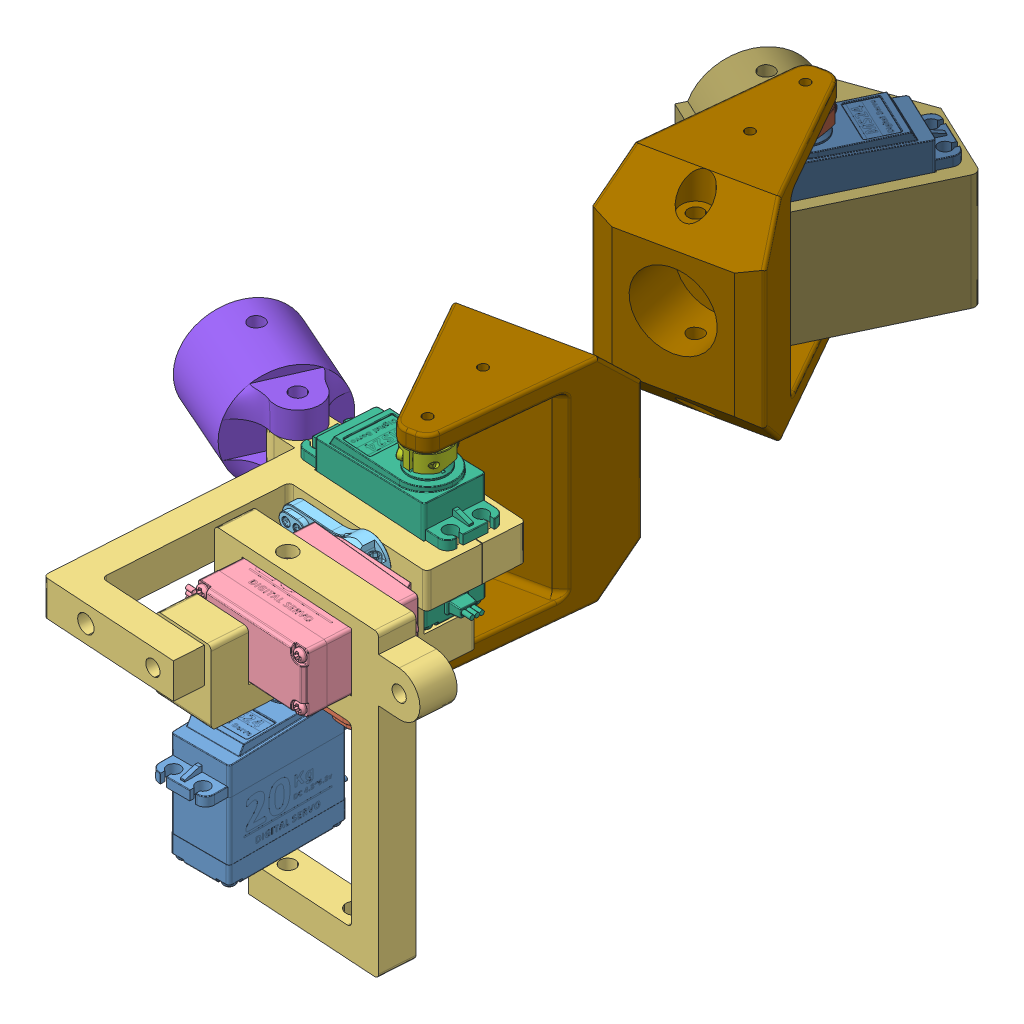
SolidWorks assembly Hip 2, configuration Default. Lengths in mm.
Overall size (141.38 121.48 305.42).
14 component instances, 12 part files, 42 mates.
Components (placement in the parent):
- Copy of DS3218MG MS24 Digital Servo 270^Hip 2-1: Copy of DS3218MG MS24 Digital Servo 270^Hip 2 [Default] at origin size (20.1 45.99 55.6) (virtual)
- Copy of Servo Arm^Hip 2-1: Copy of Servo Arm^Hip 2 [Default] x (-0.063067 0 0.998009) z (-0.998009 0 -0.063067) size (14.5 6.95 35.53) (virtual)
- Servo Connector-1: Servo Connector [Default] at (9.9951 39.015 0.6316) x (-0.998009 0 -0.063067) z (0 -1 0) size (75.07 39.5 102.5)
- Copy (3) of DS3218MG MS24 Digital Servo 270^Hip 2-1: Copy (3) of DS3218MG MS24 Digital Servo 270^Hip 2 [Default] at (0.3934 39.015 -5.9871) x (0 -1 0) z (0.998009 0 0.063067) size (20.1 45.99 55.6) (virtual)
- Copy (3) of Servo Arm^Hip 2-1: Copy (3) of Servo Arm^Hip 2 [Default] at (0.3934 39.015 -5.9871) x (0 -1 0) z (0.998009 0 0.063067) size (14.5 6.95 35.53) (virtual)
- Servo Connector-2: Servo Connector [Default] at (-7.1411 39.015 -45.5561) x (0.998009 0 0.063067) z (-0.063067 0 0.998009) size (75.07 39.5 102.5)
- Copy (2) of DS3218MG MS24 Digital Servo 270^Hip 2-1: Copy (2) of DS3218MG MS24 Digital Servo 270^Hip 2 [Default] at (2.839 45.015 -44.9254) x (-0.063067 0 0.998009) z (-0.998009 0 -0.063067) size (20.1 45.99 55.6) (virtual)
- Copy (2) of Servo Arm^Hip 2-1: Copy (2) of Servo Arm^Hip 2 [Default] at (2.839 45.015 -44.9254) x (0.978659 0 -0.205491) z (0.205491 0 0.978659) size (14.5 6.95 35.53) (virtual)
- Bar Interface-1: Bar Interface [Default] at (-60.5615 39 -54.9863) x (0 1 0) z (0.403783 0 -0.914855) size (35.43 45.1 35.43)
- Bar Attachment-3: Bar Attachment [Default] at (-5.0724 39.015 -82.6038) x (0 -1 0) z (0.205491 0 0.978659) size (72.5 49.93 66)
- Bar Attachment-4: Bar Attachment [Default] at (-23.5666 39.015 -170.6831) x (0 -1 0) z (-0.205491 0 -0.978659) size (72.5 49.93 66)
- Copy (4) of DS3218MG MS24 Digital Servo 270^Hip 2-2: Copy (4) of DS3218MG MS24 Digital Servo 270^Hip 2 [Default] at (-31.478 45.015 -208.3614) x (-0.90354 0 -0.428503) z (0.428503 0 -0.90354) size (20.1 45.99 55.6) (virtual)
- Copy (4) of Servo Arm^Hip 2-2: Copy (4) of Servo Arm^Hip 2 [Default] at (-31.478 45.015 -208.3614) x (-0.978659 0 0.205491) z (-0.205491 0 -0.978659) size (14.5 6.95 35.53) (virtual)
- Servo Connector with bar connector-3: Servo Connector with bar connector [Default] at (-27.193 39.015 -217.3968) x (-0.428503 0 0.90354) z (-0.90354 0 -0.428503) size (59.97 51.22 52.03)
Mates (geometry in assembly coordinates):
- Concentric10: concentric anti-aligned: cylinder of Copy of Servo Arm^Hip 2-1 through (0 18.4 0) axis (0 -1 0) radius 2.5; cylinder of Copy of DS3218MG MS24 Digital Servo 270^Hip 2-1 through (0 13.5 0) axis (0 1 0) radius 3.8
- Coincident5: coincident anti-aligned: plane of Copy of DS3218MG MS24 Digital Servo 270^Hip 2-1 through (0 18.4 0) normal (0 1 0); plane of Copy of Servo Arm^Hip 2-1 through (0 18.4 0) normal (0 -1 0)
- Concentric11: concentric anti-aligned: circle of Copy of Servo Arm^Hip 2-1; circle of Servo Connector-1
- Coincident6: coincident anti-aligned: plane of Copy of Servo Arm^Hip 2-1 through (9.4591 21 14.4253) normal (0 1 0); plane of Servo Connector-1 through (10.3735 21 -5.3564) normal (0 -1 0)
- Concentric1: concentric anti-aligned: cylinder of Copy (2) of Servo Arm^Hip 2-1 through (2.839 63.415 -44.9254) axis (0 -1 0) radius 2.5; cylinder of Copy (2) of DS3218MG MS24 Digital Servo 270^Hip 2-1 through (2.839 58.515 -44.9254) axis (0 1 0) radius 3.8
- Coincident1: coincident anti-aligned: plane of Copy (2) of DS3218MG MS24 Digital Servo 270^Hip 2-1 through (2.839 63.415 -44.9254) normal (0 1 0); plane of Copy (2) of Servo Arm^Hip 2-1 through (2.839 63.415 -44.9254) normal (0 -1 0)
- Concentric13: concentric anti-aligned: circle of Servo Connector-2; circle of Copy (2) of DS3218MG MS24 Digital Servo 270^Hip 2-1
- Concentric14: concentric anti-aligned: circle of Servo Connector-2; circle of Copy (2) of DS3218MG MS24 Digital Servo 270^Hip 2-1
- Coincident7: coincident anti-aligned: plane of Servo Connector-2 through (-7.1411 45.015 -45.5561) normal (0 1 0); plane of Copy (2) of DS3218MG MS24 Digital Servo 270^Hip 2-1 through (-24.6749 45.015 -37.6461) normal (0 -1 0)
- Concentric15: concentric anti-aligned: cylinder of Copy (3) of Servo Arm^Hip 2-1 through (1.5538 39.015 -24.3505) axis (-0.063067 0 0.998009) radius 2.5; cylinder of Copy (3) of DS3218MG MS24 Digital Servo 270^Hip 2-1 through (1.2448 39.015 -19.4602) axis (0.063067 0 -0.998009) radius 3.8
- Coincident8: coincident anti-aligned: plane of Copy (3) of DS3218MG MS24 Digital Servo 270^Hip 2-1 through (1.5538 39.015 -24.3505) normal (0.063067 0 -0.998009); plane of Copy (3) of Servo Arm^Hip 2-1 through (1.5538 39.015 -24.3505) normal (-0.063067 0 0.998009)
- Concentric16: concentric anti-aligned: circle of Servo Connector-1; circle of Copy (3) of DS3218MG MS24 Digital Servo 270^Hip 2-1
- Concentric17: concentric anti-aligned: circle of Servo Connector-1; circle of Copy (3) of DS3218MG MS24 Digital Servo 270^Hip 2-1
- Coincident9: coincident anti-aligned: plane of Servo Connector-1 through (10.3735 39.015 -5.3564) normal (0.063067 0 -0.998009); plane of Copy (3) of DS3218MG MS24 Digital Servo 270^Hip 2-1 through (27.3396 30.015 -4.2843) normal (-0.063067 0 0.998009)
- Concentric18: concentric anti-aligned: circle of Copy (3) of Servo Arm^Hip 2-1; circle of Servo Connector-2
- Concentric25: concentric anti-aligned: circle of Copy of Servo Arm^Hip 2-1; circle of Servo Connector-1
- Concentric26: concentric anti-aligned: circle of Servo Connector-4; circle of Servo Connector-2
- Coincident21: coincident anti-aligned: plane of Servo Connector-2 through (50.3657 5.515 -48.921) normal (0 -1 0); plane of Servo Connector-4 through (-24.9656 41.3417 -57.4873) normal (0.988432 0.123075 0.088623)
- Concentric27: concentric anti-aligned: circle of Copy (2) of Servo Arm^Hip 2-1; circle of Servo Connector-4
- Concentric35: concentric aligned: circle of Copy (2) of Servo Arm^Hip 2-1; circle of Servo Connector 2-1
- Concentric36: concentric aligned: circle of Copy (2) of Servo Arm^Hip 2-1; circle of Servo Connector 2-1
- Coincident29: coincident anti-aligned: plane of Copy (2) of Servo Arm^Hip 2-1 through (14.2176 66.015 -57.8903) normal (0 1 0); plane of Servo Connector 2-1 through (1.605 60.5411 -89.0504) normal (-0.960324 -0.044353 0.275337)
- Concentric47: concentric anti-aligned: circle of Copy of DS3218MG MS24 Digital Servo 270^Hip 2-1; circle of Servo Connector without attachment arm-2
- Concentric48: concentric anti-aligned: circle of Copy of DS3218MG MS24 Digital Servo 270^Hip 2-1; circle of Servo Connector without attachment arm-2
- Coincident34: coincident anti-aligned: plane of Copy of DS3218MG MS24 Digital Servo 270^Hip 2-1 through (9 0 27) normal (0 -1 0); plane of Servo Connector without attachment arm-2 through (0 0 10) normal (0 1 0)
- Concentric54: concentric aligned: circle of Copy (3) of Servo Arm^Hip 2-1; circle of Servo Connector-2
- Coincident38: coincident anti-aligned: plane of Copy (3) of Servo Arm^Hip 2-1 through (-8.6116 25.215 -27.598) normal (0.063067 0 -0.998009); plane of Servo Connector-2 through (-8.2773 45.015 -27.5769) normal (-0.063067 0 0.998009)
- Coincident39: coincident aligned: circle of Servo Connector-2; circle of Bar Interface-1
- Concentric55: concentric anti-aligned: circle of Copy (2) of Servo Arm^Hip 2-1; circle of Bar Attachment-3
- Concentric56: concentric aligned: circle of Copy (2) of Servo Arm^Hip 2-1; circle of Bar Attachment-3
- Coincident40: coincident anti-aligned: plane of Copy (2) of Servo Arm^Hip 2-1 through (14.2176 66.015 -57.8903) normal (0 1 0); plane of Bar Attachment-3 through (-28.5225 66.015 -71.5491) normal (0 -1 0)
- Concentric57: concentric anti-aligned: circle of Bar Attachment-3; circle of Bar Attachment-4
- Coincident42: coincident aligned: plane of Bar Attachment-3 through (-5.0724 72.015 -82.6038) normal (0 1 0); plane of Bar Attachment-4 through (-23.5666 72.015 -170.6831) normal (0 1 0)
- Concentric58: concentric anti-aligned: cylinder of Copy (4) of Servo Arm^Hip 2-2 through (-31.478 63.415 -208.3614) axis (0 -1 0) radius 2.5; cylinder of Copy (4) of DS3218MG MS24 Digital Servo 270^Hip 2-2 through (-31.478 58.515 -208.3614) axis (0 1 0) radius 3.8
- Coincident43: coincident anti-aligned: plane of Copy (4) of DS3218MG MS24 Digital Servo 270^Hip 2-2 through (-31.478 63.415 -208.3614) normal (0 1 0); plane of Copy (4) of Servo Arm^Hip 2-2 through (-31.478 63.415 -208.3614) normal (0 -1 0)
- Concentric59: concentric anti-aligned: circle of Bar Attachment-4; circle of Copy (4) of Servo Arm^Hip 2-2
- Concentric61: concentric aligned: circle of Bar Attachment-4; circle of Copy (4) of Servo Arm^Hip 2-2
- Coincident44: coincident anti-aligned: plane of Bar Attachment-4 through (-0.1165 66.015 -181.7378) normal (0 -1 0); plane of Copy (4) of Servo Arm^Hip 2-2 through (-42.8567 66.015 -195.3966) normal (0 1 0)
- Concentric62: concentric aligned: circle of Copy (4) of DS3218MG MS24 Digital Servo 270^Hip 2-2; circle of Servo Connector with bar connector-3
- Concentric63: concentric aligned: circle of Copy (4) of DS3218MG MS24 Digital Servo 270^Hip 2-2; circle of Servo Connector with bar connector-3
- Coincident45: coincident anti-aligned: plane of Copy (4) of DS3218MG MS24 Digital Servo 270^Hip 2-2 through (-28.0403 45.015 -236.6136) normal (0 -1 0); plane of Servo Connector with bar connector-3 through (-27.193 45.015 -217.3968) normal (0 1 0)
- Distance2: distance = 50 mm anti-aligned: plane of Bar Attachment-4 through (-19.4568 39.015 -151.1099) normal (0.205491 0 0.978659); plane of Bar Attachment-3 through (-9.1823 39.015 -102.1769) normal (-0.205491 0 -0.978659)
